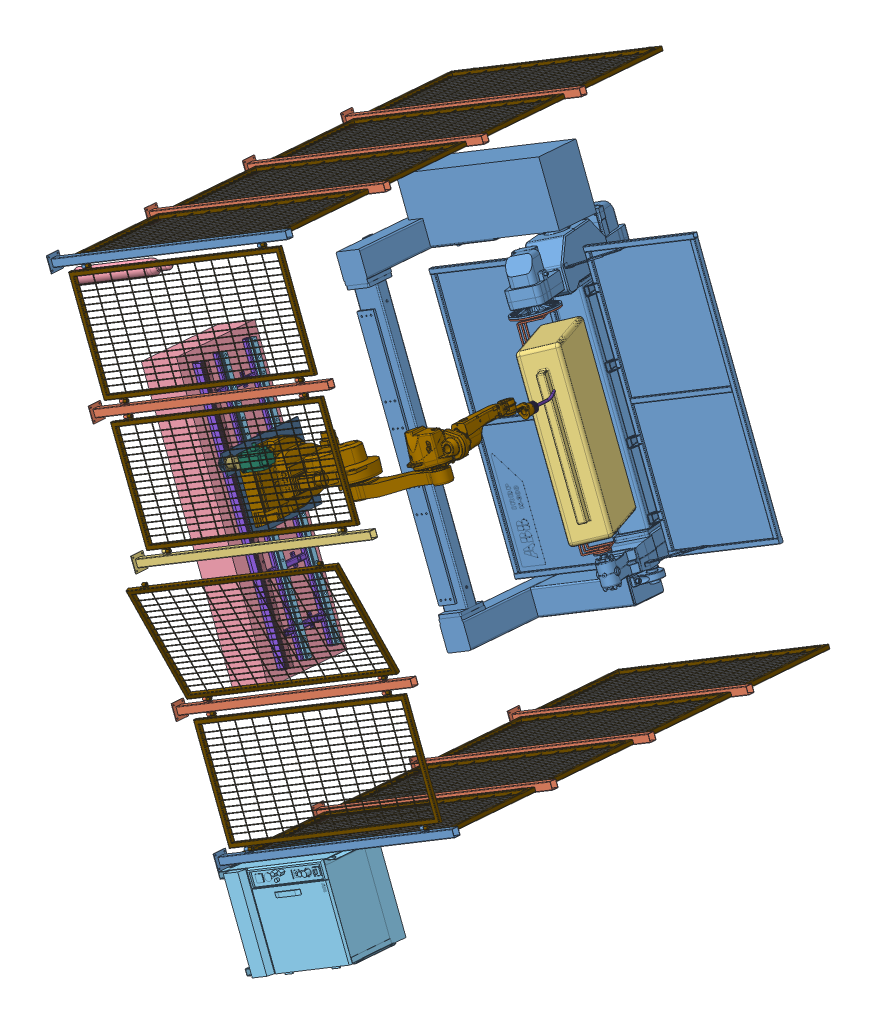
SolidWorks assembly 更新版总装图, configuration 默认. Lengths in mm.
Overall size (4498.5 5863.91 5187.28).
94 component instances, 23 part files, 16 mates.
Components (placement in the parent):
- IRBP_K300_D1000-L1600_M2009_REV1_01-1: IRBP_K300_D1000-L1600_M2009_REV1_01 [Default] at (1815.4762 156.9048 -2701.2018) x (-0.103654 -0.173243 -0.979409) z (0.478198 -0.872114 0.103654) size (1606.22 2213.46 2977)
- 变位机夹具-1: 变位机夹具 [默认] at (3149.304 377.0019 -2275.6011) x (0.478198 -0.872114 0.103654) z (0.508588 0.371205 0.776881) size (1620 350 350)
- 工件-1: 工件 [默认] at (3682.2307 -263.1434 -2305.7408) x (0.478198 -0.872114 0.103654) z (-0.716006 -0.318786 0.621056) size (1300 900 300)
- 滑轨台-1: 滑轨台 [默认] at (2486.2023 -428.863 -179.3185) x (0.478198 -0.872114 0.103654) z (0.103654 0.173243 0.979409) size (2200 300 800)
- 双导轨-2: 双导轨 [默认] at (2411.6072 -61.5883 -483.9873) x (-0.478198 0.872114 -0.103654) z (-0.103654 -0.173243 -0.979409) size (2040.11 1530 1501.91)
  - 滑轨-1: 滑轨 [默认] at (-1407.5567 207.206 0) size (2040 34 45)
  - 滑轨-2: 滑轨 [默认] at (632.4433 207.206 -300) x (-1 0 0) z (0 0 -1) size (2040 34 45)
  - 带螺钉M4滑块-1: 带螺钉M4滑块 [默认] at (-58.6161 241.6075 -300) size (138.91 46.33 120)
    - 滑块-1: 滑块 [默认] at (-71.6389 25.5985 0) size (136 46 120)
    - cross recessed round head wood screws gb-2: cross recessed round head wood screws gb [GB_WOOD_SCREWS_TYPE136 M4X18-N] at (-74.5889 20.6207 -35.126) size (20.91 7.65 7.65)
    - cross recessed round head wood screws gb-4: cross recessed round head wood screws gb [GB_WOOD_SCREWS_TYPE136 M4X18-N] at (-74.5889 -15.566 -35.2553) size (20.91 7.65 7.65)
    - cross recessed round head wood screws gb-5: cross recessed round head wood screws gb [GB_WOOD_SCREWS_TYPE136 M4X18-N] at (-74.5889 20.0027 35.5979) size (20.91 7.65 7.65)
    - cross recessed round head wood screws gb-7: cross recessed round head wood screws gb [GB_WOOD_SCREWS_TYPE136 M4X18-N] at (-74.5889 -15.4341 35.4668) size (20.91 7.65 7.65)
    - cross recessed round head wood screws gb-8: cross recessed round head wood screws gb [GB_WOOD_SCREWS_TYPE136 M4X18-N] at (56.3111 20.1247 35.1143) x (-1 0 0) z (0 -0.924225 -0.381849) size (20.91 7.65 7.65)
    - cross recessed round head wood screws gb-9: cross recessed round head wood screws gb [GB_WOOD_SCREWS_TYPE136 M4X18-N] at (56.3111 -15.3216 35.4319) x (-1 0 0) z (0 -0.924225 -0.381849) size (20.91 7.65 7.65)
    - cross recessed round head wood screws gb-10: cross recessed round head wood screws gb [GB_WOOD_SCREWS_TYPE136 M4X18-N] at (56.3111 19.9496 -35.3218) x (-1 0 0) z (0 -0.924225 -0.381849) size (20.91 7.65 7.65)
    - cross recessed round head wood screws gb-11: cross recessed round head wood screws gb [GB_WOOD_SCREWS_TYPE136 M4X18-N] at (56.3111 -15.7298 -35.1914) x (-1 0 0) z (0 -0.924225 -0.381849) size (20.91 7.65 7.65)
  - 带螺钉M4滑块-3: 带螺钉M4滑块 [默认] at (-58.6161 241.6075 0) size (138.91 46.33 120)
    - 滑块-1: 滑块 [默认] at (-71.6389 25.5985 0) size (136 46 120)
    - cross recessed round head wood screws gb-2: cross recessed round head wood screws gb [GB_WOOD_SCREWS_TYPE136 M4X18-N] at (-74.5889 20.6207 -35.126) size (20.91 7.65 7.65)
    - cross recessed round head wood screws gb-4: cross recessed round head wood screws gb [GB_WOOD_SCREWS_TYPE136 M4X18-N] at (-74.5889 -15.566 -35.2553) size (20.91 7.65 7.65)
    - cross recessed round head wood screws gb-5: cross recessed round head wood screws gb [GB_WOOD_SCREWS_TYPE136 M4X18-N] at (-74.5889 20.0027 35.5979) size (20.91 7.65 7.65)
    - cross recessed round head wood screws gb-7: cross recessed round head wood screws gb [GB_WOOD_SCREWS_TYPE136 M4X18-N] at (-74.5889 -15.4341 35.4668) size (20.91 7.65 7.65)
    - cross recessed round head wood screws gb-8: cross recessed round head wood screws gb [GB_WOOD_SCREWS_TYPE136 M4X18-N] at (56.3111 20.1247 35.1143) x (-1 0 0) z (0 -0.924225 -0.381849) size (20.91 7.65 7.65)
    - cross recessed round head wood screws gb-9: cross recessed round head wood screws gb [GB_WOOD_SCREWS_TYPE136 M4X18-N] at (56.3111 -15.3216 35.4319) x (-1 0 0) z (0 -0.924225 -0.381849) size (20.91 7.65 7.65)
    - cross recessed round head wood screws gb-10: cross recessed round head wood screws gb [GB_WOOD_SCREWS_TYPE136 M4X18-N] at (56.3111 19.9496 -35.3218) x (-1 0 0) z (0 -0.924225 -0.381849) size (20.91 7.65 7.65)
    - cross recessed round head wood screws gb-11: cross recessed round head wood screws gb [GB_WOOD_SCREWS_TYPE136 M4X18-N] at (56.3111 -15.7298 -35.1914) x (-1 0 0) z (0 -0.924225 -0.381849) size (20.91 7.65 7.65)
  - 带螺钉M4滑块-4: 带螺钉M4滑块 [默认] at (-401.8938 241.6075 0) x (-1 0 0) z (0 0 -1) size (138.91 46.33 120)
    - 滑块-1: 滑块 [默认] at (-71.6389 25.5985 0) size (136 46 120)
    - cross recessed round head wood screws gb-2: cross recessed round head wood screws gb [GB_WOOD_SCREWS_TYPE136 M4X18-N] at (-74.5889 20.6207 -35.126) size (20.91 7.65 7.65)
    - cross recessed round head wood screws gb-4: cross recessed round head wood screws gb [GB_WOOD_SCREWS_TYPE136 M4X18-N] at (-74.5889 -15.566 -35.2553) size (20.91 7.65 7.65)
    - cross recessed round head wood screws gb-5: cross recessed round head wood screws gb [GB_WOOD_SCREWS_TYPE136 M4X18-N] at (-74.5889 20.0027 35.5979) size (20.91 7.65 7.65)
    - cross recessed round head wood screws gb-7: cross recessed round head wood screws gb [GB_WOOD_SCREWS_TYPE136 M4X18-N] at (-74.5889 -15.4341 35.4668) size (20.91 7.65 7.65)
    - cross recessed round head wood screws gb-8: cross recessed round head wood screws gb [GB_WOOD_SCREWS_TYPE136 M4X18-N] at (56.3111 20.1247 35.1143) x (-1 0 0) z (0 -0.924225 -0.381849) size (20.91 7.65 7.65)
    - cross recessed round head wood screws gb-9: cross recessed round head wood screws gb [GB_WOOD_SCREWS_TYPE136 M4X18-N] at (56.3111 -15.3216 35.4319) x (-1 0 0) z (0 -0.924225 -0.381849) size (20.91 7.65 7.65)
    - cross recessed round head wood screws gb-10: cross recessed round head wood screws gb [GB_WOOD_SCREWS_TYPE136 M4X18-N] at (56.3111 19.9496 -35.3218) x (-1 0 0) z (0 -0.924225 -0.381849) size (20.91 7.65 7.65)
    - cross recessed round head wood screws gb-11: cross recessed round head wood screws gb [GB_WOOD_SCREWS_TYPE136 M4X18-N] at (56.3111 -15.7298 -35.1914) x (-1 0 0) z (0 -0.924225 -0.381849) size (20.91 7.65 7.65)
  - 带螺钉M4滑块-5: 带螺钉M4滑块 [默认] at (-401.8938 241.6075 -300) x (-1 0 0) z (0 0 -1) size (138.91 46.33 120)
    - 滑块-1: 滑块 [默认] at (-71.6389 25.5985 0) size (136 46 120)
    - cross recessed round head wood screws gb-2: cross recessed round head wood screws gb [GB_WOOD_SCREWS_TYPE136 M4X18-N] at (-74.5889 20.6207 -35.126) size (20.91 7.65 7.65)
    - cross recessed round head wood screws gb-4: cross recessed round head wood screws gb [GB_WOOD_SCREWS_TYPE136 M4X18-N] at (-74.5889 -15.566 -35.2553) size (20.91 7.65 7.65)
    - cross recessed round head wood screws gb-5: cross recessed round head wood screws gb [GB_WOOD_SCREWS_TYPE136 M4X18-N] at (-74.5889 20.0027 35.5979) size (20.91 7.65 7.65)
    - cross recessed round head wood screws gb-7: cross recessed round head wood screws gb [GB_WOOD_SCREWS_TYPE136 M4X18-N] at (-74.5889 -15.4341 35.4668) size (20.91 7.65 7.65)
    - cross recessed round head wood screws gb-8: cross recessed round head wood screws gb [GB_WOOD_SCREWS_TYPE136 M4X18-N] at (56.3111 20.1247 35.1143) x (-1 0 0) z (0 -0.924225 -0.381849) size (20.91 7.65 7.65)
    - cross recessed round head wood screws gb-9: cross recessed round head wood screws gb [GB_WOOD_SCREWS_TYPE136 M4X18-N] at (56.3111 -15.3216 35.4319) x (-1 0 0) z (0 -0.924225 -0.381849) size (20.91 7.65 7.65)
    - cross recessed round head wood screws gb-10: cross recessed round head wood screws gb [GB_WOOD_SCREWS_TYPE136 M4X18-N] at (56.3111 19.9496 -35.3218) x (-1 0 0) z (0 -0.924225 -0.381849) size (20.91 7.65 7.65)
    - cross recessed round head wood screws gb-11: cross recessed round head wood screws gb [GB_WOOD_SCREWS_TYPE136 M4X18-N] at (56.3111 -15.7298 -35.1914) x (-1 0 0) z (0 -0.924225 -0.381849) size (20.91 7.65 7.65)
  - 焊架-1: 焊架 [默认<按加工>] at (-1407.5567 174.206 -302.5) x (1 0 0) z (0 1 0) size (2040 570 90)
  - 机器人+工件台-1: 机器人+工件台 [默认] at (-235.255 279.206 -245) x (0 0 -1) z (0 1 0) size (1471.91 580 1415)
    - IRB1600ID_4_150__02_STEP_c-1: IRB1600ID_4_150__02_STEP_c [默认] at (-101.9143 0.2591 3) x (-1 0 0) z (0 0 1) size (1372.28 510.23 1392)
    - 工件台-2: 工件台 [默认] at (-50 0 -20) x (1 0 0) z (0 -1 0) size (780 23 580)
  - slotted set screws with cone point gb-18: slotted set screws with cone point gb [GB_FASTENER_SCREWS_NCOB M4X16-S] at (-90.255 263.206 -376) x (0 0 1) z (0.748487 -0.66315 0) size (15.99 4 4)
  - slotted set screws with cone point gb-16: slotted set screws with cone point gb [GB_FASTENER_SCREWS_NCOB M4X16-S] at (-30.255 263.206 -376) x (0 0 1) z (0.08595 -0.996299 0) size (15.99 4 4)
  - slotted set screws with cone point gb-15: slotted set screws with cone point gb [GB_FASTENER_SCREWS_NCOB M4X16-S] at (-50.255 263.206 -376) x (0 0 1) z (-0.998235 -0.059386 0) size (15.99 4 4)
  - slotted set screws with cone point gb-13: slotted set screws with cone point gb [GB_FASTENER_SCREWS_NCOB M4X16-S] at (-70.255 263.206 -376) x (0 0 1) z (-0.354194 -0.935172 0) size (15.99 4 4)
  - slotted set screws with cone point gb-11: slotted set screws with cone point gb [GB_FASTENER_SCREWS_NCOB M4X16-S] at (-110.255 263.206 -376) x (0 0 1) z (-0.974836 -0.222922 0) size (15.99 4 4)
  - slotted set screws with cone point gb-10: slotted set screws with cone point gb [GB_FASTENER_SCREWS_NCOB M4X16-S] at (-435.255 263.206 -376) x (0 0 1) z (-0.993007 0.118057 0) size (15.99 4 4)
  - slotted set screws with cone point gb-9: slotted set screws with cone point gb [GB_FASTENER_SCREWS_NCOB M4X16-S] at (-415.255 263.206 -376) x (0 0 1) z (-0.998721 -0.050563 0) size (15.99 4 4)
  - slotted set screws with cone point gb-7: slotted set screws with cone point gb [GB_FASTENER_SCREWS_NCOB M4X16-S] at (-395.255 263.206 -376) x (0 0 1) z (-1 0 0) size (15.99 4 4)
  - slotted set screws with cone point gb-4: slotted set screws with cone point gb [GB_FASTENER_SCREWS_NCOB M4X16-S] at (-375.255 263.206 -376) x (0 0 1) z (-0.982111 0.188301 0) size (15.99 4 4)
  - slotted set screws with cone point gb-2: slotted set screws with cone point gb [GB_FASTENER_SCREWS_NCOB M4X16-S] at (-355.255 263.206 -376) x (0 0 1) z (-0.85186 0.52377 0) size (15.99 4 4)
  - PLE8090级数2减速比15-1: PLE8090级数2减速比15 [默认] at (-22.7544 284.206 -585) x (0 -1 0) z (1 0 0) size (162.5 90 90)
  - 齿条-2: 齿条 [默认] at (-385.4567 234.206 -494) x (1 0 0) z (0 1 0) size (1018.01 46 30)
  - 齿轮-CSGH030322-2: 齿轮-CSGH030322 [默认] at (-22.7544 263.206 -585) x (0.526718 0 0.85004) z (0 -1 0) size (101.69 101.69 30)
  - 齿条-3: 齿条 [默认] at (-1403.3567 234.206 -494) x (1 0 0) z (0 1 0) size (1018.01 46 30)
  - HC-SFS1524B-1: HC-SFS1524B [默认] at (-22.7544 579.4989 -520) x (0 -1 0) z (0 0 -1) size (258 176 130)
  - 法兰盘-1: 法兰盘 [默认] at (-22.7544 430.206 -585) x (0 -1 0) z (0 0 1) size (23.5 130 130)
- 焊枪-2: 焊枪 [默认] at (3807.0352 298.3288 -1621.3147) x (0.922688 0.350908 -0.159721) z (-0.371353 0.920245 -0.123476) size (77.99 265.68 85.27)
- 防护栏装配-1: 防护栏装配 [默认] at (3597.8186 -2097.5125 1009.0072) x (-0.478198 0.872114 -0.103654) z (-0.103654 -0.173243 -0.979409) size (4807.3 2005 4351.67)
  - 150423-HL-01-02(护栏铁网856mm)-1: 150423-HL-01-02(护栏铁网856mm) [Default] at (560 1005 42.5) x (1 0 0) z (0 -1 0) size (925 35 1800)
  - 150423－HL－01－01（护拦边柱子）-1: 150423－HL－01－01（护拦边柱子） [Default] at (60 0 60) x (0 0 1) z (-1 0 0) size (124.5 2005 124.5)
  - 150423－HL－01－02（护拦柱子）-1: 150423－HL－01－02（护拦柱子） [Default] at (1060 0 60) x (0 0 1) z (-1 0 0) size (120 2005 129)
  - 150423-HL-01-02(护栏铁网856mm)-2: 150423-HL-01-02(护栏铁网856mm) [Default] at (1530.1571 1005 -102.0933) x (0.946259 0 -0.323408) z (0 -1 0) size (925 35 1800)
  - 150423－HL－01－01（护拦边柱子）-2: 150423－HL－01－01（护拦边柱子） [Default] at (4040 0 60) x (-1 0 0) z (0 0 -1) size (124.5 2005 124.5)
  - 150423-HL-01-02(护栏铁网856mm)-3: 150423-HL-01-02(护栏铁网856mm) [Default] at (3540 1005 42.5) x (1 0 0) z (0 -1 0) size (925 35 1800)
  - 150423－HL－01－02（护拦柱子）-2: 150423－HL－01－02（护拦柱子） [Default] at (3040 0 60) x (0 0 1) z (-1 0 0) size (120 2005 129)
  - 150423-HL-01-02(护栏铁网856mm)-4: 150423-HL-01-02(护栏铁网856mm) [Default] at (2539.9062 1005 45.1072) x (0.999983 0 -0.005793) z (0 -1 0) size (925 35 1800)
  - 150423－HL－01－03（护拦边柱子只一边）-1: 150423－HL－01－03（护拦边柱子只一边） [Default] at (2040.0159 0 65.5034) x (0.005793 0 0.999983) z (-0.999983 0 0.005793) size (120 2005 124.5)
  - 150423-HL-01-02(护栏铁网856mm)-5: 150423-HL-01-02(护栏铁网856mm) [Default] at (42.5 1005 560) x (0 0 -1) z (0 -1 0) size (925 35 1800)
  - 150423－HL－01－02（护拦柱子）-3: 150423－HL－01－02（护拦柱子） [Default] at (60 0 1060) size (120 2005 129)
  - 150423-HL-01-02(护栏铁网856mm)-6: 150423-HL-01-02(护栏铁网856mm) [Default] at (42.5 1005 1560) x (0 0 -1) z (0 -1 0) size (925 35 1800)
  - 150423－HL－01－02（护拦柱子）-4: 150423－HL－01－02（护拦柱子） [Default] at (60 0 2060) size (120 2005 129)
  - 150423-HL-01-02(护栏铁网856mm)-7: 150423-HL-01-02(护栏铁网856mm) [Default] at (42.5 1005 2560) x (0 0 -1) z (0 -1 0) size (925 35 1800)
  - 150423－HL－01－02（护拦柱子）-5: 150423－HL－01－02（护拦柱子） [Default] at (60 0 3060) size (120 2005 129)
  - 150423-HL-01-02(护栏铁网856mm)-8: 150423-HL-01-02(护栏铁网856mm) [Default] at (42.5 1005 3560) x (0 0 -1) z (0 -1 0) size (925 35 1800)
  - 150423-HL-01-02(护栏铁网856mm)-9: 150423-HL-01-02(护栏铁网856mm) [Default] at (4022.5 1005 1560) x (0 0 -1) z (0 -1 0) size (925 35 1800)
  - 150423-HL-01-02(护栏铁网856mm)-10: 150423-HL-01-02(护栏铁网856mm) [Default] at (4057.5 1005 560) x (0 0 1) z (0 -1 0) size (925 35 1800)
  - 150423－HL－01－02（护拦柱子）-6: 150423－HL－01－02（护拦柱子） [Default] at (4040 0 1060) size (120 2005 129)
  - 150423－HL－01－02（护拦柱子）-7: 150423－HL－01－02（护拦柱子） [Default] at (4040 0 2060) size (120 2005 129)
  - 150423-HL-01-02(护栏铁网856mm)-11: 150423-HL-01-02(护栏铁网856mm) [Default] at (4022.5 1005 2560) x (0 0 -1) z (0 -1 0) size (925 35 1800)
  - 150423－HL－01－02（护拦柱子）-8: 150423－HL－01－02（护拦柱子） [Default] at (4040 0 3060) size (120 2005 129)
  - 150423-HL-01-02(护栏铁网856mm)-12: 150423-HL-01-02(护栏铁网856mm) [Default] at (4022.5 1005 3560) x (0 0 -1) z (0 -1 0) size (925 35 1800)
  - 气瓶-1: 气瓶 [默认] at (3890.5748 0 232.4282) size (120 800 120)
  - Singel-Cabinet_IRC5_rev0-1: Singel-Cabinet_IRC5_rev0 [Default] at (-346.8 100 128.54) x (-1 0 0) z (0 0 -1) size (710.5 962.91 707.94)
Mates (geometry in assembly coordinates):
- 重合29: coincident anti-aligned: plane of IRBP_K300_D1000-L1600_M2009_REV1_01-1 through (3149.304 377.0019 -2275.6011) normal (0.478198 -0.872114 0.103654); plane of 变位机夹具-1 through (3149.304 377.0019 -2275.6011) normal (-0.478198 0.872114 -0.103654)
- 同心12: concentric aligned: cylinder of IRBP_K300_D1000-L1600_M2009_REV1_01-1 through (3129.4583 413.1955 -2279.9028) axis (0.478198 -0.872114 0.103654) radius 20; cylinder of 变位机夹具-1 through (3139.74 394.4442 -2277.6742) axis (0.478198 -0.872114 0.103654) radius 20
- 重合30: coincident anti-aligned: plane of 变位机夹具-1 through (3096.8252 317.1088 -2199.7559) normal (0.716006 0.318786 -0.621056); plane of 工件-1 through (3467.429 -358.7792 -2119.4239) normal (-0.716006 -0.318786 0.621056)
- 距离27: distance = 150 mm anti-aligned: plane of 工件-1 through (2953.1647 59.6125 -2497.5517) normal (-0.478198 0.872114 -0.103654); plane of 变位机夹具-1 through (3154.086 368.2808 -2274.5645) normal (0.478198 -0.872114 0.103654)
- 距离28: distance = 300 mm aligned: plane of 工件-1 through (3981.6932 -777.171 -1741.2961) normal (0.508588 0.371205 0.776881); plane of 变位机夹具-1 through (3271.259 403.8233 -2226.6632) normal (0.508588 0.371205 0.776881)
- 重合99: coincident anti-aligned: plane of 滑轨台-1 through (2747.8364 -291.5806 -231.2913) normal (0.872114 0.457608 -0.173243); plane of 双导轨-2/焊架-1 through (3241.818 -1170.7419 -66.7994) normal (-0.872114 -0.457608 0.173243)
- 距离35: distance = 1200 mm anti-aligned: plane of IRBP_K300_D1000-L1600_M2009_REV1_01-1 through (1867.9102 185.8644 -1856.256) normal (0.103654 0.173243 0.979409); plane of 滑轨台-1 through (3232.393 -1320.2026 -509.0354) normal (-0.103654 -0.173243 -0.979409)
- 距离37: distance = 400 mm aligned: plane of IRBP_K300_D1000-L1600_M2009_REV1_01-1 through (1623.0496 535.5324 -2554.3262) normal (-0.478198 0.872114 -0.103654); plane of 滑轨台-1 through (2263.2798 737.0413 46.4529) normal (-0.478198 0.872114 -0.103654)
- 重合105: coincident anti-aligned: plane of 双导轨-2/机器人+工件台-1/IRB1600ID_4_150__02_STEP_c-1 through (3847.2669 326.5701 -1569.3066) normal (-0.103654 -0.173243 -0.979409); plane of 焊枪-2 through (3813.2544 308.7234 -1562.5502) normal (0.103654 0.173243 0.979409)
- 同心38: concentric anti-aligned: cylinder of 双导轨-2/机器人+工件台-1/IRB1600ID_4_150__02_STEP_c-1 through (3813.7209 309.5029 -1558.1428) axis (-0.103654 -0.173243 -0.979409) radius 21; cylinder of 焊枪-2 through (3795.0841 278.3543 -1734.2385) axis (0.103654 0.173243 0.979409) radius 10
- 距离38: distance = 100 mm aligned: plane of 双导轨-2/焊架-1 through (3310.3007 -1106.2833 159.5967) normal (0.103654 0.173243 0.979409); plane of 滑轨台-1 through (3315.3163 -1181.6086 274.4921) normal (0.103654 0.173243 0.979409)
- 距离39: distance = 80 mm aligned: plane of 双导轨-2/焊架-1 through (2292.4567 622.098 -283.4513) normal (-0.478198 0.872114 -0.103654); plane of 滑轨台-1 through (2263.2798 737.0413 46.4529) normal (-0.478198 0.872114 -0.103654)
- 重合112: coincident aligned: plane of 滑轨台-1 through (2486.2023 -428.863 -179.3185) normal (-0.872114 -0.457608 0.173243); plane of 防护栏装配-1/150423－HL－01－02（护拦柱子）-4 through (3355.5991 -2402.0653 -1014.7955) normal (-0.872114 -0.457608 0.173243)
- 距离42: distance = 500 mm anti-aligned: plane of 防护栏装配-1/150423－HL－01－02（护拦柱子）-1 through (4844.5331 -297.3237 466.7452) normal (-0.103654 -0.173243 -0.979409); plane of 滑轨台-1 through (3315.3163 -1181.6086 274.4921) normal (0.103654 0.173243 0.979409)
- 距离43: distance = 400 mm anti-aligned: plane of 防护栏装配-1/150423－HL－01－01（护拦边柱子）-2 through (3425.7211 2311.9694 216.6203) normal (0.478198 -0.872114 0.103654); plane of IRBP_K300_D1000-L1600_M2009_REV1_01-1 through (1623.0496 535.5324 -2554.3262) normal (-0.478198 0.872114 -0.103654)
- 重合115: coincident aligned: plane of IRBP_K300_D1000-L1600_M2009_REV1_01-1 through (1861.4198 -5.6477 -2206.6193) normal (-0.872114 -0.457608 0.173243); plane of 滑轨台-1 through (2486.2023 -428.863 -179.3185) normal (-0.872114 -0.457608 0.173243)
